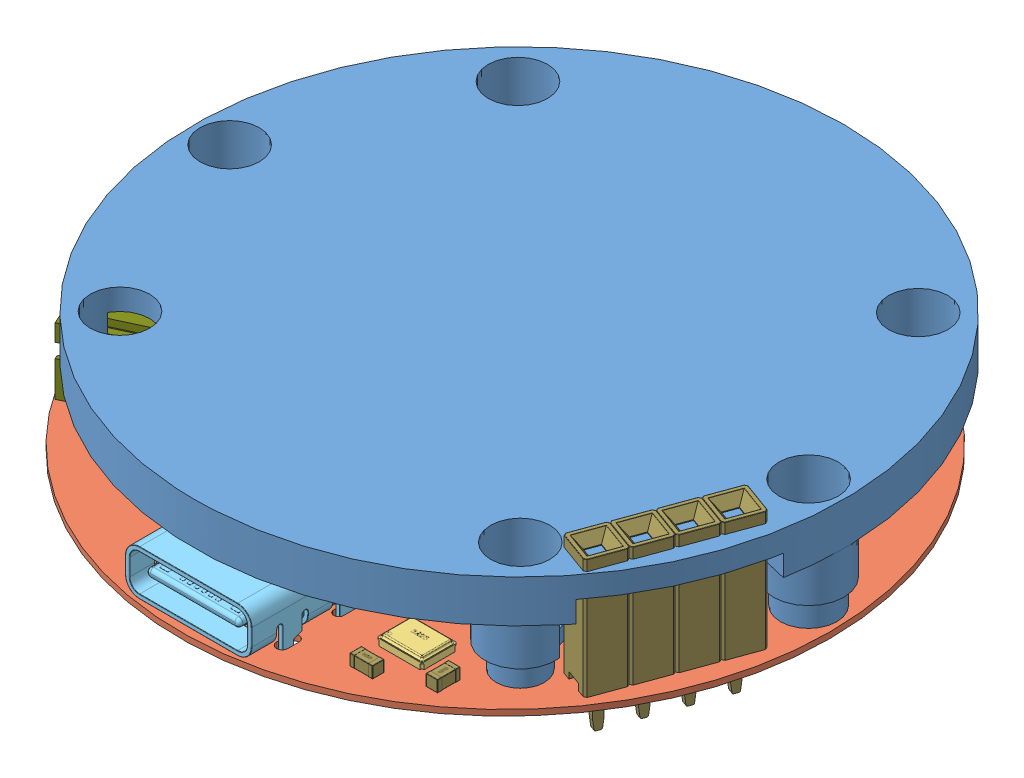
SolidWorks assembly 整体, configuration 默认. Lengths in mm.
Overall size (46.12 11.81 46.86).
340 component instances, 48 part files, 1 mates.
Components (placement in the parent):
- 4008云台电机外壳-1: 4008云台电机外壳 [默认] at (-12.9008 1.9422 46) size (46 8 46)
- STM32G4_4008_brushless_motor_pcb-1: STM32G4_4008_brushless_motor_pcb [默认] at (-104.2053 -2.8078 117.4731) x (1 0 0) z (0 1 0) size (46 46 11.81)
  - STM32G4_4008_brushless_motor_pcb.step-1: STM32G4_4008_brushless_motor_pcb.step [默认] at origin size (46 46 11.81)
    - Board.step-1: Board.step [默认] at origin size (46 46 0.41)
      - Open CASCADE STEP translator 6.8 1.1.1.step-1: Open CASCADE STEP translator 6.8 1.1.1.step [默认] at (0 0 -0.4115) size (46 46 0.41)
    - X1.step-1: X1.step [默认] at origin size (3.2 2.5 0.72)
      - OSC_3225-4.step-1: OSC_3225-4.step [默认] at (100.5332 55.0164 0) size (3.2 2.5 0.72)
        - OSC_3225-4-0.step-1: OSC_3225-4-0.step [默认] at origin size (3.2 2.5 0.72)
        - LOGO_0.15.step-1: LOGO_0.15.step [默认] at (-0.0166 0.0115 -0.003) size (0.45 0.52 0)
    - USB1.step-1: USB1.step [默认] at origin size (8.94 7.9 4.1)
      - USB_Type-C_A.step-1: USB_Type-C_A.step [默认] at (91.2368 50.7239 0) x (-1 0 0) z (0 0 1) size (8.94 7.9 4.1)
        - USB_Type-C_A-1.step-1: USB_Type-C_A-1.step [默认] at origin size (8.94 7.9 4.1)
        - LOGO_0.5.step-1: LOGO_0.5.step [默认] at (0.0308 -0.1109 0.04) size (1.5 1.73 0.01)
    - U7.step-1: U7.step [默认] at origin size (6.5 7.02 1.67)
      - SOT223.step-1: SOT223.step [默认] at (75.7682 73.3044 0) size (6.5 7.02 1.67)
        - SOT223-2.step-1: SOT223-2.step [默认] at origin size (6.5 3.5 1.6)
        - SOT223___-1.step-1: SOT223___-1.step [默认] at (0 1.75 0.725) size (3 1.76 0.92)
        - SOT223___-2.step-1: SOT223___-2.step [默认] at (2.3 -1.75 0.725) x (-1 0 0) z (0 0 1) size (0.71 1.76 0.92)
        - SOT223___-2.step-2: SOT223___-2.step [默认] at (0 -1.75 0.725) x (-1 0 0) z (0 0 1) size (0.71 1.76 0.92)
        - SOT223___-2.step-3: SOT223___-2.step [默认] at (-2.3 -1.75 0.725) x (-1 0 0) z (0 0 1) size (0.71 1.76 0.92)
        - LOGO_0.25.step-1: LOGO_0.25.step [默认] at origin size (0.75 0.87 0.01)
    - U6.step-1: U6.step [默认] at origin size (9 9 1.05)
      - TQFP48_7x7.step-1: TQFP48_7x7.step [默认] at (100.9904 65.4812 0) x (-1 0 0) z (0 0 1) size (9 9 1.05)
        - TQFP48_7x7______.step-1: TQFP48_7x7______.step [默认] at origin size (7 7 1)
        - _____0.25.step-1: _____0.25.step [默认] at (2.75 -3.5 0.55) x (-1 0 0) z (0 0 1) size (0.25 1 0.6)
        - _____0.25.step-2: _____0.25.step [默认] at (2.25 -3.5 0.55) x (-1 0 0) z (0 0 1) size (0.25 1 0.6)
        - _____0.25.step-3: _____0.25.step [默认] at (1.75 -3.5 0.55) x (-1 0 0) z (0 0 1) size (0.25 1 0.6)
        - _____0.25.step-4: _____0.25.step [默认] at (1.25 -3.5 0.55) x (-1 0 0) z (0 0 1) size (0.25 1 0.6)
        - _____0.25.step-5: _____0.25.step [默认] at (0.75 -3.5 0.55) x (-1 0 0) z (0 0 1) size (0.25 1 0.6)
        - _____0.25.step-6: _____0.25.step [默认] at (0.25 -3.5 0.55) x (-1 0 0) z (0 0 1) size (0.25 1 0.6)
        - _____0.25.step-7: _____0.25.step [默认] at (-0.25 -3.5 0.55) x (-1 0 0) z (0 0 1) size (0.25 1 0.6)
        - _____0.25.step-8: _____0.25.step [默认] at (-0.75 -3.5 0.55) x (-1 0 0) z (0 0 1) size (0.25 1 0.6)
        - _____0.25.step-9: _____0.25.step [默认] at (-1.25 -3.5 0.55) x (-1 0 0) z (0 0 1) size (0.25 1 0.6)
        - _____0.25.step-10: _____0.25.step [默认] at (-1.75 -3.5 0.55) x (-1 0 0) z (0 0 1) size (0.25 1 0.6)
        - _____0.25.step-11: _____0.25.step [默认] at (-2.25 -3.5 0.55) x (-1 0 0) z (0 0 1) size (0.25 1 0.6)
        - _____0.25.step-12: _____0.25.step [默认] at (-2.75 -3.5 0.55) x (-1 0 0) z (0 0 1) size (0.25 1 0.6)
        - _____0.25.step-13: _____0.25.step [默认] at (3.5 2.75 0.55) x (0 -1 0) z (0 0 1) size (0.25 1 0.6)
        - _____0.25.step-14: _____0.25.step [默认] at (-2.75 3.5 0.55) size (0.25 1 0.6)
        - _____0.25.step-15: _____0.25.step [默认] at (-3.5 -2.75 0.55) x (0 1 0) z (0 0 1) size (0.25 1 0.6)
        - _____0.25.step-16: _____0.25.step [默认] at (3.5 2.25 0.55) x (0 -1 0) z (0 0 1) size (0.25 1 0.6)
        - _____0.25.step-17: _____0.25.step [默认] at (-2.25 3.5 0.55) size (0.25 1 0.6)
        - _____0.25.step-18: _____0.25.step [默认] at (-3.5 -2.25 0.55) x (0 1 0) z (0 0 1) size (0.25 1 0.6)
        - _____0.25.step-19: _____0.25.step [默认] at (3.5 1.75 0.55) x (0 -1 0) z (0 0 1) size (0.25 1 0.6)
        - _____0.25.step-20: _____0.25.step [默认] at (-1.75 3.5 0.55) size (0.25 1 0.6)
        - _____0.25.step-21: _____0.25.step [默认] at (-3.5 -1.75 0.55) x (0 1 0) z (0 0 1) size (0.25 1 0.6)
        - _____0.25.step-22: _____0.25.step [默认] at (3.5 1.25 0.55) x (0 -1 0) z (0 0 1) size (0.25 1 0.6)
        - _____0.25.step-23: _____0.25.step [默认] at (-1.25 3.5 0.55) size (0.25 1 0.6)
        - _____0.25.step-24: _____0.25.step [默认] at (-3.5 -1.25 0.55) x (0 1 0) z (0 0 1) size (0.25 1 0.6)
        - _____0.25.step-25: _____0.25.step [默认] at (3.5 0.75 0.55) x (0 -1 0) z (0 0 1) size (0.25 1 0.6)
        - _____0.25.step-26: _____0.25.step [默认] at (-0.75 3.5 0.55) size (0.25 1 0.6)
        - _____0.25.step-27: _____0.25.step [默认] at (-3.5 -0.75 0.55) x (0 1 0) z (0 0 1) size (0.25 1 0.6)
        - _____0.25.step-28: _____0.25.step [默认] at (3.5 0.25 0.55) x (0 -1 0) z (0 0 1) size (0.25 1 0.6)
        - _____0.25.step-29: _____0.25.step [默认] at (-0.25 3.5 0.55) size (0.25 1 0.6)
        - _____0.25.step-30: _____0.25.step [默认] at (-3.5 -0.25 0.55) x (0 1 0) z (0 0 1) size (0.25 1 0.6)
        - _____0.25.step-31: _____0.25.step [默认] at (3.5 -0.25 0.55) x (0 -1 0) z (0 0 1) size (0.25 1 0.6)
        - _____0.25.step-32: _____0.25.step [默认] at (0.25 3.5 0.55) size (0.25 1 0.6)
        - _____0.25.step-33: _____0.25.step [默认] at (-3.5 0.25 0.55) x (0 1 0) z (0 0 1) size (0.25 1 0.6)
        - _____0.25.step-34: _____0.25.step [默认] at (3.5 -0.75 0.55) x (0 -1 0) z (0 0 1) size (0.25 1 0.6)
        - _____0.25.step-35: _____0.25.step [默认] at (0.75 3.5 0.55) size (0.25 1 0.6)
        - _____0.25.step-36: _____0.25.step [默认] at (-3.5 0.75 0.55) x (0 1 0) z (0 0 1) size (0.25 1 0.6)
        - _____0.25.step-37: _____0.25.step [默认] at (3.5 -1.25 0.55) x (0 -1 0) z (0 0 1) size (0.25 1 0.6)
        - _____0.25.step-38: _____0.25.step [默认] at (1.25 3.5 0.55) size (0.25 1 0.6)
        - _____0.25.step-39: _____0.25.step [默认] at (-3.5 1.25 0.55) x (0 1 0) z (0 0 1) size (0.25 1 0.6)
        - _____0.25.step-40: _____0.25.step [默认] at (3.5 -1.75 0.55) x (0 -1 0) z (0 0 1) size (0.25 1 0.6)
        - _____0.25.step-41: _____0.25.step [默认] at (1.75 3.5 0.55) size (0.25 1 0.6)
        - _____0.25.step-42: _____0.25.step [默认] at (-3.5 1.75 0.55) x (0 1 0) z (0 0 1) size (0.25 1 0.6)
        - _____0.25.step-43: _____0.25.step [默认] at (3.5 -2.25 0.55) x (0 -1 0) z (0 0 1) size (0.25 1 0.6)
        - _____0.25.step-44: _____0.25.step [默认] at (2.25 3.5 0.55) size (0.25 1 0.6)
        - _____0.25.step-45: _____0.25.step [默认] at (-3.5 2.25 0.55) x (0 1 0) z (0 0 1) size (0.25 1 0.6)
        - _____0.25.step-46: _____0.25.step [默认] at (3.5 -2.75 0.55) x (0 -1 0) z (0 0 1) size (0.25 1 0.6)
        - _____0.25.step-47: _____0.25.step [默认] at (2.75 3.5 0.55) size (0.25 1 0.6)
        - _____0.25.step-48: _____0.25.step [默认] at (-3.5 2.75 0.55) x (0 1 0) z (0 0 1) size (0.25 1 0.6)
        - LOGO_0.25-3.step-1: LOGO_0.25-3.step [默认] at (0.012 -0.0139 0.045) size (0.75 0.87 0.01)
    - U5.step-1: U5.step [默认] at origin size (3 2.81 1.18)
      - SOT23-6.step-1: SOT23-6.step [默认] at (85.3693 63.043 0) x (-1 0 0) z (0 0 1) size (3 2.81 1.18)
        - SOT23-5and6_____.step-1: SOT23-5and6_____.step [默认] at (-0.95 -0.8 0.675) x (-1 0 0) z (0 0 1) size (0.4 0.6 0.78)
        - SOT23-5and6_____.step-2: SOT23-5and6_____.step [默认] at (0 -0.8 0.675) x (-1 0 0) z (0 0 1) size (0.4 0.6 0.78)
        - SOT23-5and6_____.step-3: SOT23-5and6_____.step [默认] at (0.95 -0.8 0.675) x (-1 0 0) z (0 0 1) size (0.4 0.6 0.78)
        - SOT23-5and6_____.step-4: SOT23-5and6_____.step [默认] at (-0.95 0.8 0.675) size (0.4 0.6 0.78)
        - SOT23-5and6_____.step-5: SOT23-5and6_____.step [默认] at (0.95 0.8 0.675) size (0.4 0.6 0.78)
        - LOGO_0.15-4.step-1: LOGO_0.15-4.step [默认] at (0 -0.0167 0.0485) x (-1 0 0) z (0 0 -1) size (0.45 0.52 0)
        - SOT23-6-5.step-1: SOT23-6-5.step [默认] at origin size (3 1.6 1.1)
        - SOT23-5and6_____.step-6: SOT23-5and6_____.step [默认] at (0 0.8 0.675) size (0.4 0.6 0.78)
    - U4.step-1: U4.step [默认] at origin size (2.2 2.4 1.1)
      - User_Library-SOT363-2.step-1: User_Library-SOT363-2.step [默认] at (83.9827 82.123 0) x (-1 0 0) z (0 0 1) size (2.2 2.4 1.1)
    - U3.step-1: U3.step [默认] at origin size (2.2 2.4 1.1)
      - User_Library-SOT363-2.step-1: User_Library-SOT363-2.step [默认] at (88.3815 82.2404 0) x (-1 0 0) z (0 0 1) size (2.2 2.4 1.1)
    - U2.step-1: U2.step [默认] at origin size (6.01 5 1.9)
      - SOP8.step-1: SOP8.step [默认] at (91.186 70.612 -0.4115) x (-1 0 0) z (0 0 -1) size (6.01 5 1.9)
        - LOGO_0.25-6.step-1: LOGO_0.25-6.step [默认] at (0.0116 0 0.095) x (0 -1 0) z (0 0 -1) size (0.75 0.87 0.01)
        - SOP8_____.step-1: SOP8_____.step [默认] at origin size (3.6 5 1.8)
        - ____1.8_______.step-1: ____1.8_______.step [默认] at (1.8 1.91 1) x (0 1 0) z (0 0 1) size (0.5 1.2 1.1)
        - ____1.8_______.step-2: ____1.8_______.step [默认] at (1.8 0.64 1) x (0 1 0) z (0 0 1) size (0.5 1.2 1.1)
        - ____1.8_______.step-3: ____1.8_______.step [默认] at (1.8 -0.63 1) x (0 1 0) z (0 0 1) size (0.5 1.2 1.1)
        - ____1.8_______.step-4: ____1.8_______.step [默认] at (1.8 -1.9 1) x (0 1 0) z (0 0 1) size (0.5 1.2 1.1)
        - ____1.8_______.step-5: ____1.8_______.step [默认] at (-1.8 1.91 1) x (0 -1 0) z (0 0 1) size (0.5 1.2 1.1)
        - ____1.8_______.step-6: ____1.8_______.step [默认] at (-1.8 0.64 1) x (0 -1 0) z (0 0 1) size (0.5 1.2 1.1)
        - ____1.8_______.step-7: ____1.8_______.step [默认] at (-1.8 -0.63 1) x (0 -1 0) z (0 0 1) size (0.5 1.2 1.1)
        - ____1.8_______.step-8: ____1.8_______.step [默认] at (-1.8 -1.9 1) x (0 -1 0) z (0 0 1) size (0.5 1.2 1.1)
    - U1.step-1: U1.step [默认] at origin size (9.8 6.4 1.05)
      - TSSOP28.step-1: TSSOP28.step [默认] at (102.9208 78.3336 0) x (0 -1 0) z (0 0 1) size (6.4 9.8 1.05)
        - TSSOP28_____.step-1: TSSOP28_____.step [默认] at origin size (4.6 9.8 1)
        - _____0.9.step-1: _____0.9.step [默认] at (-2.3 4.225 0.53) x (0 -1 0) z (0 0 1) size (0.25 0.9 0.6)
        - _____0.9.step-2: _____0.9.step [默认] at (-2.3 3.575 0.53) x (0 -1 0) z (0 0 1) size (0.25 0.9 0.6)
        - _____0.9.step-3: _____0.9.step [默认] at (-2.3 2.925 0.53) x (0 -1 0) z (0 0 1) size (0.25 0.9 0.6)
        - _____0.9.step-4: _____0.9.step [默认] at (-2.3 2.275 0.53) x (0 -1 0) z (0 0 1) size (0.25 0.9 0.6)
        - _____0.9.step-5: _____0.9.step [默认] at (-2.3 1.625 0.53) x (0 -1 0) z (0 0 1) size (0.25 0.9 0.6)
        - _____0.9.step-6: _____0.9.step [默认] at (-2.3 0.975 0.53) x (0 -1 0) z (0 0 1) size (0.25 0.9 0.6)
        - _____0.9.step-7: _____0.9.step [默认] at (-2.3 0.325 0.53) x (0 -1 0) z (0 0 1) size (0.25 0.9 0.6)
        - _____0.9.step-8: _____0.9.step [默认] at (-2.3 -0.325 0.53) x (0 -1 0) z (0 0 1) size (0.25 0.9 0.6)
        - _____0.9.step-9: _____0.9.step [默认] at (-2.3 -0.975 0.53) x (0 -1 0) z (0 0 1) size (0.25 0.9 0.6)
        - _____0.9.step-10: _____0.9.step [默认] at (-2.3 -1.625 0.53) x (0 -1 0) z (0 0 1) size (0.25 0.9 0.6)
        - _____0.9.step-11: _____0.9.step [默认] at (-2.3 -2.275 0.53) x (0 -1 0) z (0 0 1) size (0.25 0.9 0.6)
        - _____0.9.step-12: _____0.9.step [默认] at (-2.3 -2.925 0.53) x (0 -1 0) z (0 0 1) size (0.25 0.9 0.6)
        - _____0.9.step-13: _____0.9.step [默认] at (-2.3 -3.575 0.53) x (0 -1 0) z (0 0 1) size (0.25 0.9 0.6)
        - _____0.9.step-14: _____0.9.step [默认] at (-2.3 -4.225 0.53) x (0 -1 0) z (0 0 1) size (0.25 0.9 0.6)
        - _____0.9.step-15: _____0.9.step [默认] at (2.3 4.225 0.53) x (0 1 0) z (0 0 1) size (0.25 0.9 0.6)
        - _____0.9.step-16: _____0.9.step [默认] at (2.3 3.575 0.53) x (0 1 0) z (0 0 1) size (0.25 0.9 0.6)
        - _____0.9.step-17: _____0.9.step [默认] at (2.3 2.925 0.53) x (0 1 0) z (0 0 1) size (0.25 0.9 0.6)
        - _____0.9.step-18: _____0.9.step [默认] at (2.3 2.275 0.53) x (0 1 0) z (0 0 1) size (0.25 0.9 0.6)
        - _____0.9.step-19: _____0.9.step [默认] at (2.3 1.625 0.53) x (0 1 0) z (0 0 1) size (0.25 0.9 0.6)
        - _____0.9.step-20: _____0.9.step [默认] at (2.3 0.975 0.53) x (0 1 0) z (0 0 1) size (0.25 0.9 0.6)
        - _____0.9.step-21: _____0.9.step [默认] at (2.3 0.325 0.53) x (0 1 0) z (0 0 1) size (0.25 0.9 0.6)
        - _____0.9.step-22: _____0.9.step [默认] at (2.3 -0.325 0.53) x (0 1 0) z (0 0 1) size (0.25 0.9 0.6)
        - _____0.9.step-23: _____0.9.step [默认] at (2.3 -0.975 0.53) x (0 1 0) z (0 0 1) size (0.25 0.9 0.6)
        - _____0.9.step-24: _____0.9.step [默认] at (2.3 -1.625 0.53) x (0 1 0) z (0 0 1) size (0.25 0.9 0.6)
        - _____0.9.step-25: _____0.9.step [默认] at (2.3 -2.275 0.53) x (0 1 0) z (0 0 1) size (0.25 0.9 0.6)
        - _____0.9.step-26: _____0.9.step [默认] at (2.3 -2.925 0.53) x (0 1 0) z (0 0 1) size (0.25 0.9 0.6)
        - _____0.9.step-27: _____0.9.step [默认] at (2.3 -3.575 0.53) x (0 1 0) z (0 0 1) size (0.25 0.9 0.6)
        - _____0.9.step-28: _____0.9.step [默认] at (2.3 -4.225 0.53) x (0 1 0) z (0 0 1) size (0.25 0.9 0.6)
        - LOGO_0.25-7.step-1: LOGO_0.25-7.step [默认] at (0 0.1751 0.025) size (0.75 0.87 0.01)
    - R16.step-1: R16.step [默认] at origin size (1.6 0.8 0.41)
      - R_0603-HP.step-1: R_0603-HP.step [默认] at (103.3526 58.9789 -0.4115) x (-1 0 0) z (0 0 -1) size (1.6 0.8 0.4)
        - R_0603.step-1: R_0603.step [默认] at origin size (1.6 0.8 0.4)
        - LOGO_.step-1: LOGO_.step [默认] at (0.0001 0.0322 -0.002) x (-1 0 0) z (0 0 -1) size (0.6 0.69 0)
    - R15.step-1: R15.step [默认] at origin size (0.8 1.6 0.4)
      - R_0603-HP.step-1: R_0603-HP.step [默认] at (96.1897 73.2536 0) x (0 1 0) z (0 0 1) size (1.6 0.8 0.4)
        - R_0603.step-1: R_0603.step [默认] at origin size (1.6 0.8 0.4)
        - LOGO_.step-1: LOGO_.step [默认] at (0.0001 0.0322 -0.002) x (-1 0 0) z (0 0 -1) size (0.6 0.69 0)
    - R14.step-1: R14.step [默认] at origin size (0.8 1.6 0.4)
      - R_0603-HP.step-1: R_0603-HP.step [默认] at (96.1389 76.5048 0) x (0 1 0) z (0 0 1) size (1.6 0.8 0.4)
        - R_0603.step-1: R_0603.step [默认] at origin size (1.6 0.8 0.4)
        - LOGO_.step-1: LOGO_.step [默认] at (0.0001 0.0322 -0.002) x (-1 0 0) z (0 0 -1) size (0.6 0.69 0)
    - R13.step-1: R13.step [默认] at origin size (1.6 0.8 0.4)
      - R_0603-HP.step-1: R_0603-HP.step [默认] at (92.6234 64.8969 0) x (-1 0 0) z (0 0 1) size (1.6 0.8 0.4)
        - R_0603.step-1: R_0603.step [默认] at origin size (1.6 0.8 0.4)
        - LOGO_.step-1: LOGO_.step [默认] at (0.0001 0.0322 -0.002) x (-1 0 0) z (0 0 -1) size (0.6 0.69 0)
    - R12.step-1: R12.step [默认] at origin size (0.8 1.6 0.41)
      - R_0603-HP.step-1: R_0603-HP.step [默认] at (97.2313 60.8688 -0.4115) x (0 1 0) z (0 0 -1) size (1.6 0.8 0.4)
        - R_0603.step-1: R_0603.step [默认] at origin size (1.6 0.8 0.4)
        - LOGO_.step-1: LOGO_.step [默认] at (0.0001 0.0322 -0.002) x (-1 0 0) z (0 0 -1) size (0.6 0.69 0)
    - R11.step-1: R11.step [默认] at origin size (0.8 1.6 0.41)
      - R_0603-HP.step-1: R_0603-HP.step [默认] at (95.0215 60.8688 -0.4115) x (0 1 0) z (0 0 -1) size (1.6 0.8 0.4)
        - R_0603.step-1: R_0603.step [默认] at origin size (1.6 0.8 0.4)
        - LOGO_.step-1: LOGO_.step [默认] at (0.0001 0.0322 -0.002) x (-1 0 0) z (0 0 -1) size (0.6 0.69 0)
    - R10.step-1: R10.step [默认] at origin size (0.8 1.6 0.41)
      - R_0603-HP.step-1: R_0603-HP.step [默认] at (92.8117 60.8688 -0.4115) x (0 1 0) z (0 0 -1) size (1.6 0.8 0.4)
        - R_0603.step-1: R_0603.step [默认] at origin size (1.6 0.8 0.4)
        - LOGO_.step-1: LOGO_.step [默认] at (0.0001 0.0322 -0.002) x (-1 0 0) z (0 0 -1) size (0.6 0.69 0)
    - R9.step-1: R9.step [默认] at origin size (1.6 0.8 0.4)
      - R_0603-HP.step-1: R_0603-HP.step [默认] at (85.979 84.6835 0) x (-1 0 0) z (0 0 1) size (1.6 0.8 0.4)
        - R_0603.step-1: R_0603.step [默认] at origin size (1.6 0.8 0.4)
        - LOGO_.step-1: LOGO_.step [默认] at (0.0001 0.0322 -0.002) x (-1 0 0) z (0 0 -1) size (0.6 0.69 0)
    - R8.step-1: R8.step [默认] at origin size (6.4 3.2 0.57)
      - R_2512-HP.step-1: R_2512-HP.step [默认] at (85.7758 88.5953 0) x (1 0 0) z (0 0 1) size (6.4 3.2 0.57)
        - R_2512.step-1: R_2512.step [默认] at origin size (6.4 3.2 0.55)
        - LOGO_-8.step-1: LOGO_-8.step [默认] at (-0.005 0.1842 -0.008) x (-1 0 0) z (0 0 -1) size (2.4 2.77 0.02)
    - R7.step-1: R7.step [默认] at origin size (0.8 1.6 0.4)
      - R_0603-HP.step-1: R_0603-HP.step [默认] at (81.7373 83.7334 0) x (0 -1 0) z (0 0 1) size (1.6 0.8 0.4)
        - R_0603.step-1: R_0603.step [默认] at origin size (1.6 0.8 0.4)
        - LOGO_.step-1: LOGO_.step [默认] at (0.0001 0.0322 -0.002) x (-1 0 0) z (0 0 -1) size (0.6 0.69 0)
    - R6.step-1: R6.step [默认] at origin size (0.8 1.6 0.4)
      - R_0603-HP.step-1: R_0603-HP.step [默认] at (90.7541 80.264 0) x (0 1 0) z (0 0 1) size (1.6 0.8 0.4)
        - R_0603.step-1: R_0603.step [默认] at origin size (1.6 0.8 0.4)
        - LOGO_.step-1: LOGO_.step [默认] at (0.0001 0.0322 -0.002) x (-1 0 0) z (0 0 -1) size (0.6 0.69 0)
    - R5.step-1: R5.step [默认] at origin size (1.6 0.8 0.41)
      - R_0603-HP.step-1: R_0603-HP.step [默认] at (89.1898 66.2179 -0.4115) x (-1 0 0) z (0 0 -1) size (1.6 0.8 0.4)
        - R_0603.step-1: R_0603.step [默认] at origin size (1.6 0.8 0.4)
        - LOGO_.step-1: LOGO_.step [默认] at (0.0001 0.0322 -0.002) x (-1 0 0) z (0 0 -1) size (0.6 0.69 0)
    - R4.step-1: R4.step [默认] at origin size (6.4 3.2 0.57)
      - R_2512-HP.step-1: R_2512-HP.step [默认] at (85.8521 76.4795 0) x (1 0 0) z (0 0 1) size (6.4 3.2 0.57)
        - R_2512.step-1: R_2512.step [默认] at origin size (6.4 3.2 0.55)
        - LOGO_-8.step-1: LOGO_-8.step [默认] at (-0.005 0.1842 -0.008) x (-1 0 0) z (0 0 -1) size (2.4 2.77 0.02)
    - R3.step-1: R3.step [默认] at origin size (0.8 1.6 0.4)
      - R_0603-HP.step-1: R_0603-HP.step [默认] at (86.2329 80.3402 0) x (0 1 0) z (0 0 1) size (1.6 0.8 0.4)
        - R_0603.step-1: R_0603.step [默认] at origin size (1.6 0.8 0.4)
        - LOGO_.step-1: LOGO_.step [默认] at (0.0001 0.0322 -0.002) x (-1 0 0) z (0 0 -1) size (0.6 0.69 0)
    - R2.step-1: R2.step [默认] at origin size (0.8 1.6 0.41)
      - R_0603-HP.step-1: R_0603-HP.step [默认] at (84.5567 72.0956 -0.4115) x (0 1 0) z (0 0 -1) size (1.6 0.8 0.4)
        - R_0603.step-1: R_0603.step [默认] at origin size (1.6 0.8 0.4)
        - LOGO_.step-1: LOGO_.step [默认] at (0.0001 0.0322 -0.002) x (-1 0 0) z (0 0 -1) size (0.6 0.69 0)
    - R1.step-1: R1.step [默认] at origin size (0.8 1.6 0.41)
      - R_0603-HP.step-1: R_0603-HP.step [默认] at (84.5565 68.5695 -0.4115) x (0 -1 0) z (0 0 -1) size (1.6 0.8 0.4)
        - R_0603.step-1: R_0603.step [默认] at origin size (1.6 0.8 0.4)
        - LOGO_.step-1: LOGO_.step [默认] at (0.0001 0.0322 -0.002) x (-1 0 0) z (0 0 -1) size (0.6 0.69 0)
    - L1.step-1: L1.step [默认] at origin size (6.95 6.6 3.03)
      - SMD-0630.step-1: SMD-0630.step [默认] at (86.1314 70.104 0) x (-1 0 0) z (0 0 1) size (6.95 6.6 3.03)
        - SMD-0630-9.step-1: SMD-0630-9.step [默认] at origin size (6.95 6.6 3.03)
        - LOGO_0.5-10.step-1: LOGO_0.5-10.step [默认] at (0 0.0017 0.04) size (1.5 1.73 0.01)
    - J3.step-1: J3.step [默认] at origin size (5.86 10.42 11.5)
      - HDR2.54-1P_M.step-1: HDR2.54-1P_M.step [默认] at (109.7 61.824 0) x (0.34202 0.939693 0) z (0 0 1) size (2.54 2.54 11.5)
        - HDR2.54-1P_M-11.step-1: HDR2.54-1P_M-11.step [默认] at origin size (2.54 2.54 11.5)
        - LOGO_-12.step-1: LOGO_-12.step [默认] at (0 0.9721 0.0285) x (-1 0 0) z (0 0 -1) size (0.45 0.52 0)
      - HDR2.54-1P_M.step-2: HDR2.54-1P_M.step [默认] at (108.8313 59.4372 0) x (0.34202 0.939693 0) z (0 0 1) size (2.54 2.54 11.5)
        - HDR2.54-1P_M-11.step-1: HDR2.54-1P_M-11.step [默认] at origin size (2.54 2.54 11.5)
        - LOGO_-12.step-1: LOGO_-12.step [默认] at (0 0.9721 0.0285) x (-1 0 0) z (0 0 -1) size (0.45 0.52 0)
      - HDR2.54-1P_M.step-3: HDR2.54-1P_M.step [默认] at (111.4375 66.5976 0) x (0.34202 0.939693 0) z (0 0 1) size (2.54 2.54 11.5)
        - HDR2.54-1P_M-11.step-1: HDR2.54-1P_M-11.step [默认] at origin size (2.54 2.54 11.5)
        - LOGO_-12.step-1: LOGO_-12.step [默认] at (0 0.9721 0.0285) x (-1 0 0) z (0 0 -1) size (0.45 0.52 0)
      - HDR2.54-1P_M.step-4: HDR2.54-1P_M.step [默认] at (110.5688 64.2108 0) x (0.34202 0.939693 0) z (0 0 1) size (2.54 2.54 11.5)
        - HDR2.54-1P_M-11.step-1: HDR2.54-1P_M-11.step [默认] at origin size (2.54 2.54 11.5)
        - LOGO_-12.step-1: LOGO_-12.step [默认] at (0 0.9721 0.0285) x (-1 0 0) z (0 0 -1) size (0.45 0.52 0)
    - J2.step-1: J2.step [默认] at origin size (9.32 9.95 7.4)
      - PH2.0-WI-3P.step-1: PH2.0-WI-3P.step [默认] at (76.581 63.627 0) x (0.422618 -0.906308 0) z (0 0 1) size (7.9 6.6 7.4)
        - PH2.0-WI-____.step-1: PH2.0-WI-____.step [默认] at (-2 0 0.05) size (0.6 5.5 6)
        - PH2.0-WI-____.step-2: PH2.0-WI-____.step [默认] at (0 0 0.05) size (0.6 5.5 6)
        - LOGO_0.25-13.step-1: LOGO_0.25-13.step [默认] at (-0.0263 -2.2762 0.045) size (0.75 0.87 0.01)
        - PH2.0-WI-____.step-3: PH2.0-WI-____.step [默认] at (2 0 0.05) size (0.6 5.5 6)
        - PH2.0-WI-3P-14.step-1: PH2.0-WI-3P-14.step [默认] at origin size (7.9 6 4.7)
    - J1.step-1: J1.step [默认] at origin size (5 4.95 2.9)
      - 3D_Model.step-1: 3D_Model.step [默认] at (79.8815 81.6977 -0.4115) x (-1 0 0) z (0 -1 0) size (5 2.9 4.95)
        - SH_1_0-LT-3P_ASM_1_AF0_ASM.step-1: SH_1_0-LT-3P_ASM_1_AF0_ASM.step [默认] at origin size (5 2.9 4.95)
          - ID20001_ASM_1_AF0_ASM_1_AF0_ASM.step-1: ID20001_ASM_1_AF0_ASM_1_AF0_ASM.step [默认] at origin size (5 2.9 4.95)
            - 3DID1_AF00001_ASM_1_AF0_ASM_1_ASM.step-1: 3DID1_AF00001_ASM_1_AF0_ASM_1_ASM.step [默认] at origin size (3.6 2.9 4.95)
              - LPATTERN3_11__1_AF0_1_1_1_2.step-1: LPATTERN3_11__1_AF0_1_1_1_2.step [默认] at origin size (0.2 2.4 1.2)
              - LPATTERN3_7__1_3_1.step-1: LPATTERN3_7__1_3_1.step [默认] at origin size (0.2 2.4 1.2)
              - LPATTERN3_2__1_3_1.step-1: LPATTERN3_2__1_3_1.step [默认] at origin size (0.2 2.4 1.2)
              - LPATTERN3_6__1_AF0_3_1.step-1: LPATTERN3_6__1_AF0_3_1.step [默认] at origin size (0.2 2.4 1.2)
              - EXTRUDE8_1_1_1.step-1: EXTRUDE8_1_1_1.step [默认] at origin size (0.3 1.25 1.5)
              - PIN_1_MARK_1_AF0_3_AF0_1.step-1: PIN_1_MARK_1_AF0_3_AF0_1.step [默认] at origin size (3.6 2.8 4.25)
              - LPATTERN3_3__1_1_1.step-1: LPATTERN3_3__1_1_1.step [默认] at origin size (0.2 2.4 1.2)
              - LPATTERN3_1__1_AF0_3_1.step-1: LPATTERN3_1__1_AF0_3_1.step [默认] at origin size (0.2 2.4 1.2)
            - SH1_0-2L_ASM_1_AF0_ASM_1_AF0_ASM.step-1: SH1_0-2L_ASM_1_AF0_ASM_1_AF0_ASM.step [默认] at (-3 0 0) size (1.4 2.9 4.25)
              - ID0001_ASM_1_ASM_1_AF0_ASM_1_AF0_ASM.step-1: ID0001_ASM_1_ASM_1_AF0_ASM_1_AF0_ASM.step [默认] at origin size (1.4 2.9 4.25)
                - EXTRUDE7_1_1_1_1_AF0.step-1: EXTRUDE7_1_1_1_1_AF0.step [默认] at origin size (0.3 1.25 1.5)
                - PIN_1_MARK_AF0_1_1_AF0_1.step-1: PIN_1_MARK_AF0_1_1_AF0_1.step [默认] at origin size (1.4 2.8 4.25)
    - D2.step-1: D2.step [默认] at origin size (2.6 5.12 2.11)
      - SMA.step-1: SMA.step [默认] at (93.3957 73.7591 0.05) x (0 -1 0) z (0 0 1) size (5.12 2.6 2.11)
        - SMA-15.step-1: SMA-15.step [默认] at origin size (5.12 2.6 2.1)
        - LOGO______.__.step-1: LOGO______.__.step [默认] at (0.0018 0.0048 -0.003) x (-1 0 0) z (0 0 -1) size (0.9 1.04 0.01)
    - D1.step-1: D1.step [默认] at origin size (2.6 5.12 2.11)
      - SMA.step-1: SMA.step [默认] at (82.7531 56.1315 0.05) x (0 -1 0) z (0 0 1) size (5.12 2.6 2.11)
        - SMA-15.step-1: SMA-15.step [默认] at origin size (5.12 2.6 2.1)
        - LOGO______.__.step-1: LOGO______.__.step [默认] at (0.0018 0.0048 -0.003) x (-1 0 0) z (0 0 -1) size (0.9 1.04 0.01)
    - C24.step-1: C24.step [默认] at origin size (1.6 0.82 0.82)
      - C_0603.step-1: C_0603.step [默认] at (78.9686 67.0306 0) x (1 0 0) z (0 0 1) size (1.6 0.82 0.82)
        - LOGO_-16.step-1: LOGO_-16.step [默认] at (0 0.0171 -0.0006) x (-1 0 0) z (0 0 -1) size (0.51 0.59 0)
        - C_0603-17.step-1: C_0603-17.step [默认] at origin size (1.6 0.82 0.82)
    - C23.step-1: C23.step [默认] at origin size (1.6 0.82 0.82)
      - C_0603.step-1: C_0603.step [默认] at (75.0824 80.1116 0) x (1 0 0) z (0 0 1) size (1.6 0.82 0.82)
        - LOGO_-16.step-1: LOGO_-16.step [默认] at (0 0.0171 -0.0006) x (-1 0 0) z (0 0 -1) size (0.51 0.59 0)
        - C_0603-17.step-1: C_0603-17.step [默认] at origin size (1.6 0.82 0.82)
    - C22.step-1: C22.step [默认] at origin size (1.6 0.82 0.82)
      - C_0603.step-1: C_0603.step [默认] at (103.3526 60.5282 -0.4115) x (1 0 0) z (0 0 -1) size (1.6 0.82 0.82)
        - LOGO_-16.step-1: LOGO_-16.step [默认] at (0 0.0171 -0.0006) x (-1 0 0) z (0 0 -1) size (0.51 0.59 0)
        - C_0603-17.step-1: C_0603-17.step [默认] at origin size (1.6 0.82 0.82)
    - C21.step-1: C21.step [默认] at origin size (0.82 1.6 0.82)
      - C_0603.step-1: C_0603.step [默认] at (82.0674 62.5602 0) x (0 1 0) z (0 0 1) size (1.6 0.82 0.82)
        - LOGO_-16.step-1: LOGO_-16.step [默认] at (0 0.0171 -0.0006) x (-1 0 0) z (0 0 -1) size (0.51 0.59 0)
        - C_0603-17.step-1: C_0603-17.step [默认] at origin size (1.6 0.82 0.82)
    - C20.step-1: C20.step [默认] at origin size (0.82 1.6 0.82)
      - C_0603.step-1: C_0603.step [默认] at (103.632 53.7568 0) x (0 -1 0) z (0 0 1) size (1.6 0.82 0.82)
        - LOGO_-16.step-1: LOGO_-16.step [默认] at (0 0.0171 -0.0006) x (-1 0 0) z (0 0 -1) size (0.51 0.59 0)
        - C_0603-17.step-1: C_0603-17.step [默认] at origin size (1.6 0.82 0.82)
    - C19.step-1: C19.step [默认] at origin size (1.6 0.82 0.82)
      - C_0603.step-1: C_0603.step [默认] at (94.0816 78.2066 0) x (1 0 0) z (0 0 1) size (1.6 0.82 0.82)
        - LOGO_-16.step-1: LOGO_-16.step [默认] at (0 0.0171 -0.0006) x (-1 0 0) z (0 0 -1) size (0.51 0.59 0)
        - C_0603-17.step-1: C_0603-17.step [默认] at origin size (1.6 0.82 0.82)
    - C18.step-1: C18.step [默认] at origin size (0.82 1.6 0.82)
      - C_0603.step-1: C_0603.step [默认] at (107.6452 68.4276 0) x (0 -1 0) z (0 0 1) size (1.6 0.82 0.82)
        - LOGO_-16.step-1: LOGO_-16.step [默认] at (0 0.0171 -0.0006) x (-1 0 0) z (0 0 -1) size (0.51 0.59 0)
        - C_0603-17.step-1: C_0603-17.step [默认] at origin size (1.6 0.82 0.82)
    - C17.step-1: C17.step [默认] at origin size (0.82 1.6 0.82)
      - C_0603.step-1: C_0603.step [默认] at (93.345 62.611 0) x (0 1 0) z (0 0 1) size (1.6 0.82 0.82)
        - LOGO_-16.step-1: LOGO_-16.step [默认] at (0 0.0171 -0.0006) x (-1 0 0) z (0 0 -1) size (0.51 0.59 0)
        - C_0603-17.step-1: C_0603-17.step [默认] at origin size (1.6 0.82 0.82)
    - C16.step-1: C16.step [默认] at origin size (0.82 1.6 0.82)
      - C_0603.step-1: C_0603.step [默认] at (107.6198 64.8866 0) x (0 -1 0) z (0 0 1) size (1.6 0.82 0.82)
        - LOGO_-16.step-1: LOGO_-16.step [默认] at (0 0.0171 -0.0006) x (-1 0 0) z (0 0 -1) size (0.51 0.59 0)
        - C_0603-17.step-1: C_0603-17.step [默认] at origin size (1.6 0.82 0.82)
    - C15.step-1: C15.step [默认] at origin size (1.6 0.82 0.82)
      - C_0603.step-1: C_0603.step [默认] at (98.8314 72.6186 0) x (1 0 0) z (0 0 1) size (1.6 0.82 0.82)
        - LOGO_-16.step-1: LOGO_-16.step [默认] at (0 0.0171 -0.0006) x (-1 0 0) z (0 0 -1) size (0.51 0.59 0)
        - C_0603-17.step-1: C_0603-17.step [默认] at origin size (1.6 0.82 0.82)
    - C14.step-1: C14.step [默认] at origin size (1.6 0.82 0.82)
      - C_0603.step-1: C_0603.step [默认] at (100.0864 51.9176 0) x (1 0 0) z (0 0 1) size (1.6 0.82 0.82)
        - LOGO_-16.step-1: LOGO_-16.step [默认] at (0 0.0171 -0.0006) x (-1 0 0) z (0 0 -1) size (0.51 0.59 0)
        - C_0603-17.step-1: C_0603-17.step [默认] at origin size (1.6 0.82 0.82)
    - C13.step-1: C13.step [默认] at origin size (0.82 1.6 0.82)
      - C_0603.step-1: C_0603.step [默认] at (79.7814 83.693 0) x (0 1 0) z (0 0 1) size (1.6 0.82 0.82)
        - LOGO_-16.step-1: LOGO_-16.step [默认] at (0 0.0171 -0.0006) x (-1 0 0) z (0 0 -1) size (0.51 0.59 0)
        - C_0603-17.step-1: C_0603-17.step [默认] at origin size (1.6 0.82 0.82)
    - C12.step-1: C12.step [默认] at origin size (1.6 0.82 0.82)
      - C_0603.step-1: C_0603.step [默认] at (101.9914 72.6186 -0.4115) x (1 0 0) z (0 0 -1) size (1.6 0.82 0.82)
        - LOGO_-16.step-1: LOGO_-16.step [默认] at (0 0.0171 -0.0006) x (-1 0 0) z (0 0 -1) size (0.51 0.59 0)
        - C_0603-17.step-1: C_0603-17.step [默认] at origin size (1.6 0.82 0.82)
    - C11.step-1: C11.step [默认] at origin size (0.82 1.6 0.82)
      - C_0603.step-1: C_0603.step [默认] at (100.6958 86.995 0) x (0 1 0) z (0 0 1) size (1.6 0.82 0.82)
        - LOGO_-16.step-1: LOGO_-16.step [默认] at (0 0.0171 -0.0006) x (-1 0 0) z (0 0 -1) size (0.51 0.59 0)
        - C_0603-17.step-1: C_0603-17.step [默认] at origin size (1.6 0.82 0.82)
    - C10.step-1: C10.step [默认] at origin size (0.82 1.6 0.82)
      - C_0603.step-1: C_0603.step [默认] at (93.4212 86.995 0) x (0 1 0) z (0 0 1) size (1.6 0.82 0.82)
        - LOGO_-16.step-1: LOGO_-16.step [默认] at (0 0.0171 -0.0006) x (-1 0 0) z (0 0 -1) size (0.51 0.59 0)
        - C_0603-17.step-1: C_0603-17.step [默认] at origin size (1.6 0.82 0.82)
    - C9.step-1: C9.step [默认] at origin size (0.82 1.6 0.82)
      - C_0603.step-1: C_0603.step [默认] at (95.2399 86.995 0) x (0 1 0) z (0 0 1) size (1.6 0.82 0.82)
        - LOGO_-16.step-1: LOGO_-16.step [默认] at (0 0.0171 -0.0006) x (-1 0 0) z (0 0 -1) size (0.51 0.59 0)
        - C_0603-17.step-1: C_0603-17.step [默认] at origin size (1.6 0.82 0.82)
    - C8.step-1: C8.step [默认] at origin size (0.82 1.6 0.82)
      - C_0603.step-1: C_0603.step [默认] at (97.0585 86.995 0) x (0 1 0) z (0 0 1) size (1.6 0.82 0.82)
        - LOGO_-16.step-1: LOGO_-16.step [默认] at (0 0.0171 -0.0006) x (-1 0 0) z (0 0 -1) size (0.51 0.59 0)
        - C_0603-17.step-1: C_0603-17.step [默认] at origin size (1.6 0.82 0.82)
    - C7.step-1: C7.step [默认] at origin size (0.82 1.6 0.82)
      - C_0603.step-1: C_0603.step [默认] at (98.8771 86.995 0) x (0 1 0) z (0 0 1) size (1.6 0.82 0.82)
        - LOGO_-16.step-1: LOGO_-16.step [默认] at (0 0.0171 -0.0006) x (-1 0 0) z (0 0 -1) size (0.51 0.59 0)
        - C_0603-17.step-1: C_0603-17.step [默认] at origin size (1.6 0.82 0.82)
    - C6.step-1: C6.step [默认] at origin size (0.82 1.6 0.82)
      - C_0603.step-1: C_0603.step [默认] at (90.7288 83.5152 0) x (0 1 0) z (0 0 1) size (1.6 0.82 0.82)
        - LOGO_-16.step-1: LOGO_-16.step [默认] at (0 0.0171 -0.0006) x (-1 0 0) z (0 0 -1) size (0.51 0.59 0)
        - C_0603-17.step-1: C_0603-17.step [默认] at origin size (1.6 0.82 0.82)
    - C5.step-1: C5.step [默认] at origin size (0.82 1.6 0.82)
      - C_0603.step-1: C_0603.step [默认] at (97.0788 70.0278 -0.4115) x (0 -1 0) z (0 0 -1) size (1.6 0.82 0.82)
        - LOGO_-16.step-1: LOGO_-16.step [默认] at (0 0.0171 -0.0006) x (-1 0 0) z (0 0 -1) size (0.51 0.59 0)
        - C_0603-17.step-1: C_0603-17.step [默认] at origin size (1.6 0.82 0.82)
    - C4.step-1: C4.step [默认] at origin size (0.82 1.6 0.82)
      - C_0603.step-1: C_0603.step [默认] at (99.2378 70.0278 -0.4115) x (0 -1 0) z (0 0 -1) size (1.6 0.82 0.82)
        - LOGO_-16.step-1: LOGO_-16.step [默认] at (0 0.0171 -0.0006) x (-1 0 0) z (0 0 -1) size (0.51 0.59 0)
        - C_0603-17.step-1: C_0603-17.step [默认] at origin size (1.6 0.82 0.82)
    - C3.step-1: C3.step [默认] at origin size (1.6 0.82 0.82)
      - C_0603.step-1: C_0603.step [默认] at (104.8004 87.122 0) x (-1 0 0) z (0 0 1) size (1.6 0.82 0.82)
        - LOGO_-16.step-1: LOGO_-16.step [默认] at (0 0.0171 -0.0006) x (-1 0 0) z (0 0 -1) size (0.51 0.59 0)
        - C_0603-17.step-1: C_0603-17.step [默认] at origin size (1.6 0.82 0.82)
    - C2.step-1: C2.step [默认] at origin size (0.82 1.6 0.82)
      - C_0603.step-1: C_0603.step [默认] at (102.5144 86.995 0) x (0 -1 0) z (0 0 1) size (1.6 0.82 0.82)
        - LOGO_-16.step-1: LOGO_-16.step [默认] at (0 0.0171 -0.0006) x (-1 0 0) z (0 0 -1) size (0.51 0.59 0)
        - C_0603-17.step-1: C_0603-17.step [默认] at origin size (1.6 0.82 0.82)
    - C1.step-1: C1.step [默认] at origin size (1.6 0.82 0.82)
      - C_0603.step-1: C_0603.step [默认] at (107.2134 78.5876 -0.4115) x (-1 0 0) z (0 0 -1) size (1.6 0.82 0.82)
        - LOGO_-16.step-1: LOGO_-16.step [默认] at (0 0.0171 -0.0006) x (-1 0 0) z (0 0 -1) size (0.51 0.59 0)
        - C_0603-17.step-1: C_0603-17.step [默认] at origin size (1.6 0.82 0.82)
Mates (geometry in assembly coordinates):
- 重合1: coincident anti-aligned: plane of 4008云台电机外壳-1 through (-12.9008 1.9422 46) normal (0 -1 0); plane of STM32G4_4008_brushless_motor_pcb-1/STM32G4_4008_brushless_motor_pcb.step-1/J2.step-1/PH2.0-WI-3P.step-1/PH2.0-WI-3P-14.step-1 through (-27.6243 1.9422 53.8461) normal (0 1 0)
